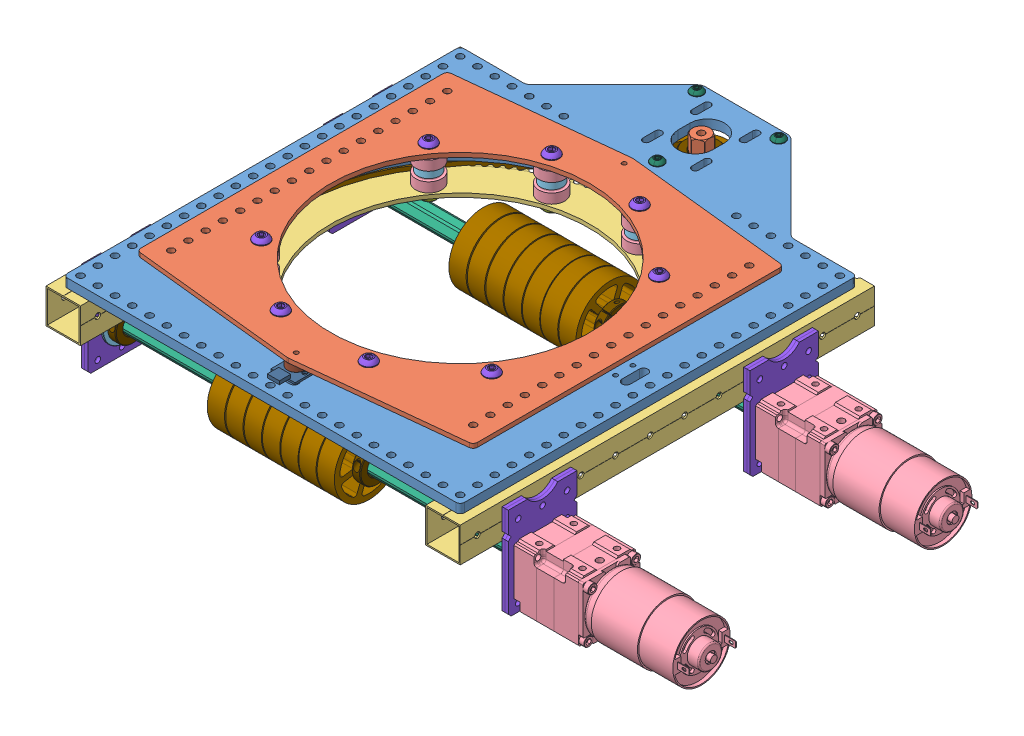
SolidWorks assembly Turret, configuration Default. Lengths in mm.
Overall size (762 1050.2 1114.79).
152 component instances, 28 part files, 7 mates.
Components (placement in the parent):
- Skeleton-1: Skeleton [Default] at origin
- WCP-0280 Rev1 - GreyT Turret-1: WCP-0280 Rev1 - GreyT Turret [Default] at (0 538.7787 -157.715) size (454.1 179.88 363.61)
  - WCP-0280-001 Rev1-1: WCP-0280-001 Rev1 [Default] at origin size (292.1 6.6 356.64)
  - spinner_tray_+_sprocket^WCP-0280 Rev1 - GreyT Turret-1: spinner_tray_+_sprocket^WCP-0280 Rev1 - GreyT Turret [Default] at origin size (248.55 39.23 334.09)
    - WCP-0280-002 Rev1-1: WCP-0280-002 Rev1 [Default] at (0 12.9476 0) size (247.65 3.17 254)
    - WCP-0280-004 Rev1-1: WCP-0280-004 Rev1 [Default] at (0 -14.1605 0) size (246.3 3.25 246.3)
    - bearing_assembly^spinner_tray_+_sprocket-1: bearing_assembly^spinner_tray_+_sprocket [Default] at (-31.5529 25.185 -41.3287) size (26.53 39.23 26.53)
      - WCP-0212_0_250_radial_bearing-1: WCP-0212_0_250_radial_bearing [Default] at (-53.2118 -18.2653 102.9139) x (-0.999427 0 0.033839) z (0 -1 0) size (19.05 19.05 7.14)
      - WCP-0212_0_250_radial_bearing-2: WCP-0212_0_250_radial_bearing [Default] at (-53.2118 -32.1147 102.9139) x (-0.572891 0 0.819632) z (0 1 0) size (19.05 19.05 7.14)
      - WCP-0041_0_250_radial_bearing-1: WCP-0041_0_250_radial_bearing [Default] at (-53.2118 -25.19 102.9139) x (-0.872331 0 0.488916) z (0 -1 0) size (15.88 15.88 4.98)
      - NFS-0011_0_250ID_fiber_washer_95601A310-1: NFS-0011_0_250ID_fiber_washer_95601A310 [Default] at (-53.2118 -35.6866 102.9139) x (0 -1 0) z (-0.326131 0 -0.945325) size (0.86 9.53 9.53)
      - NFS-0011_0_250ID_fiber_washer_95601A310-2: NFS-0011_0_250ID_fiber_washer_95601A310 [Default] at (-53.2118 -22.7008 102.9139) x (0 1 0) z (-0.943269 0 0.332029) size (0.86 9.53 9.53)
      - NFS-0011_0_250ID_fiber_washer_95601A310-3: NFS-0011_0_250ID_fiber_washer_95601A310 [Default] at (-53.2118 -28.5428 102.9139) x (0 1 0) z (-0.160822 0 -0.986983) size (0.86 9.53 9.53)
      - NFS-0011_0_250ID_fiber_washer_95601A310-4: NFS-0011_0_250ID_fiber_washer_95601A310 [Default] at (-53.2118 -14.6935 102.9139) x (0 1 0) z (-0.168532 0 -0.985696) size (0.86 9.53 9.53)
      - NFS-0024_250-20_thin_locknut_90566A029-1: NFS-0024_250-20_thin_locknut_90566A029 [Default] at (-53.2118 -39.3502 102.9139) x (0.28034 0 -0.959901) z (-0.959901 0 -0.28034) size (11.11 5.35 12.83)
      - NFS-0057_SHCS_250-20_1_375L_91255A526-1: NFS-0057_SHCS_250-20_1_375L_91255A526 [Default] at (-53.2118 -7.2971 102.9139) x (0.67695 0 0.736029) z (0 1 0) size (11.17 11.22 39.23)
    - WCP-0280-005 Rev1-1: WCP-0280-005 Rev1 [Default] at (0 -12.7603 -88.6925) size (248.55 9 320.83)
    - hall_effect_board_WCP-0971-1: hall_effect_board_WCP-0971 [Default] at (-8.89 3.302 116.459) x (-1 0 0) z (0 1 0) size (17.78 21.08 5.08)
    - hall_effect_magnet_WCP-0030-1: hall_effect_magnet_WCP-0030 [Default] at (0 8.8602 120.65) x (0.543179 0 0.839617) z (-0.839617 0 0.543179) size (12.7 5 12.7)
    - bearing_assembly^spinner_tray_+_sprocket-2: bearing_assembly^spinner_tray_+_sprocket [Default] at (-51.901 25.185 -172.6831) x (0.982082 0 -0.188455) z (0.188455 0 0.982082) size (26.53 39.23 26.53)
      - WCP-0212_0_250_radial_bearing-1: WCP-0212_0_250_radial_bearing [Default] at (-53.2118 -18.2653 102.9139) x (-0.999427 0 0.033839) z (0 -1 0) size (19.05 19.05 7.14)
      - WCP-0212_0_250_radial_bearing-2: WCP-0212_0_250_radial_bearing [Default] at (-53.2118 -32.1147 102.9139) x (-0.572891 0 0.819632) z (0 1 0) size (19.05 19.05 7.14)
      - WCP-0041_0_250_radial_bearing-1: WCP-0041_0_250_radial_bearing [Default] at (-53.2118 -25.19 102.9139) x (-0.872331 0 0.488916) z (0 -1 0) size (15.88 15.88 4.98)
      - NFS-0011_0_250ID_fiber_washer_95601A310-1: NFS-0011_0_250ID_fiber_washer_95601A310 [Default] at (-53.2118 -35.6866 102.9139) x (0 -1 0) z (-0.326131 0 -0.945325) size (0.86 9.53 9.53)
      - NFS-0011_0_250ID_fiber_washer_95601A310-2: NFS-0011_0_250ID_fiber_washer_95601A310 [Default] at (-53.2118 -22.7008 102.9139) x (0 1 0) z (-0.943269 0 0.332029) size (0.86 9.53 9.53)
      - NFS-0011_0_250ID_fiber_washer_95601A310-3: NFS-0011_0_250ID_fiber_washer_95601A310 [Default] at (-53.2118 -28.5428 102.9139) x (0 1 0) z (-0.160822 0 -0.986983) size (0.86 9.53 9.53)
      - NFS-0011_0_250ID_fiber_washer_95601A310-4: NFS-0011_0_250ID_fiber_washer_95601A310 [Default] at (-53.2118 -14.6935 102.9139) x (0 1 0) z (-0.168532 0 -0.985696) size (0.86 9.53 9.53)
      - NFS-0024_250-20_thin_locknut_90566A029-1: NFS-0024_250-20_thin_locknut_90566A029 [Default] at (-53.2118 -39.3502 102.9139) x (0.28034 0 -0.959901) z (-0.959901 0 -0.28034) size (11.11 5.35 12.83)
      - NFS-0057_SHCS_250-20_1_375L_91255A526-1: NFS-0057_SHCS_250-20_1_375L_91255A526 [Default] at (-53.2118 -7.2971 102.9139) x (0.67695 0 0.736029) z (0 1 0) size (11.17 11.22 39.23)
    - bearing_assembly^spinner_tray_+_sprocket-3: bearing_assembly^spinner_tray_+_sprocket [Default] at (-24.2359 25.185 -215.2172) x (0.918365 0 -0.395734) z (0.395734 0 0.918365) size (26.53 39.23 26.53)
      - WCP-0212_0_250_radial_bearing-1: WCP-0212_0_250_radial_bearing [Default] at (-53.2118 -18.2653 102.9139) x (-0.999427 0 0.033839) z (0 -1 0) size (19.05 19.05 7.14)
      - WCP-0212_0_250_radial_bearing-2: WCP-0212_0_250_radial_bearing [Default] at (-53.2118 -32.1147 102.9139) x (-0.572891 0 0.819632) z (0 1 0) size (19.05 19.05 7.14)
      - WCP-0041_0_250_radial_bearing-1: WCP-0041_0_250_radial_bearing [Default] at (-53.2118 -25.19 102.9139) x (-0.872331 0 0.488916) z (0 -1 0) size (15.88 15.88 4.98)
      - NFS-0011_0_250ID_fiber_washer_95601A310-1: NFS-0011_0_250ID_fiber_washer_95601A310 [Default] at (-53.2118 -35.6866 102.9139) x (0 -1 0) z (-0.326131 0 -0.945325) size (0.86 9.53 9.53)
      - NFS-0011_0_250ID_fiber_washer_95601A310-2: NFS-0011_0_250ID_fiber_washer_95601A310 [Default] at (-53.2118 -22.7008 102.9139) x (0 1 0) z (-0.943269 0 0.332029) size (0.86 9.53 9.53)
      - NFS-0011_0_250ID_fiber_washer_95601A310-3: NFS-0011_0_250ID_fiber_washer_95601A310 [Default] at (-53.2118 -28.5428 102.9139) x (0 1 0) z (-0.160822 0 -0.986983) size (0.86 9.53 9.53)
      - NFS-0011_0_250ID_fiber_washer_95601A310-4: NFS-0011_0_250ID_fiber_washer_95601A310 [Default] at (-53.2118 -14.6935 102.9139) x (0 1 0) z (-0.168532 0 -0.985696) size (0.86 9.53 9.53)
      - NFS-0024_250-20_thin_locknut_90566A029-1: NFS-0024_250-20_thin_locknut_90566A029 [Default] at (-53.2118 -39.3502 102.9139) x (0.28034 0 -0.959901) z (-0.959901 0 -0.28034) size (11.11 5.35 12.83)
      - NFS-0057_SHCS_250-20_1_375L_91255A526-1: NFS-0057_SHCS_250-20_1_375L_91255A526 [Default] at (-53.2118 -7.2971 102.9139) x (0.67695 0 0.736029) z (0 1 0) size (11.17 11.22 39.23)
    - bearing_assembly^spinner_tray_+_sprocket-4: bearing_assembly^spinner_tray_+_sprocket [Default] at (13.1984 25.185 -213.9052) x (0.8 0 -0.6) z (0.6 0 0.8) size (26.53 39.23 26.53)
      - WCP-0212_0_250_radial_bearing-1: WCP-0212_0_250_radial_bearing [Default] at (-53.2118 -18.2653 102.9139) x (-0.999427 0 0.033839) z (0 -1 0) size (19.05 19.05 7.14)
      - WCP-0212_0_250_radial_bearing-2: WCP-0212_0_250_radial_bearing [Default] at (-53.2118 -32.1147 102.9139) x (-0.572891 0 0.819632) z (0 1 0) size (19.05 19.05 7.14)
      - WCP-0041_0_250_radial_bearing-1: WCP-0041_0_250_radial_bearing [Default] at (-53.2118 -25.19 102.9139) x (-0.872331 0 0.488916) z (0 -1 0) size (15.88 15.88 4.98)
      - NFS-0011_0_250ID_fiber_washer_95601A310-1: NFS-0011_0_250ID_fiber_washer_95601A310 [Default] at (-53.2118 -35.6866 102.9139) x (0 -1 0) z (-0.326131 0 -0.945325) size (0.86 9.53 9.53)
      - NFS-0011_0_250ID_fiber_washer_95601A310-2: NFS-0011_0_250ID_fiber_washer_95601A310 [Default] at (-53.2118 -22.7008 102.9139) x (0 1 0) z (-0.943269 0 0.332029) size (0.86 9.53 9.53)
      - NFS-0011_0_250ID_fiber_washer_95601A310-3: NFS-0011_0_250ID_fiber_washer_95601A310 [Default] at (-53.2118 -28.5428 102.9139) x (0 1 0) z (-0.160822 0 -0.986983) size (0.86 9.53 9.53)
      - NFS-0011_0_250ID_fiber_washer_95601A310-4: NFS-0011_0_250ID_fiber_washer_95601A310 [Default] at (-53.2118 -14.6935 102.9139) x (0 1 0) z (-0.168532 0 -0.985696) size (0.86 9.53 9.53)
      - NFS-0024_250-20_thin_locknut_90566A029-1: NFS-0024_250-20_thin_locknut_90566A029 [Default] at (-53.2118 -39.3502 102.9139) x (0.28034 0 -0.959901) z (-0.959901 0 -0.28034) size (11.11 5.35 12.83)
      - NFS-0057_SHCS_250-20_1_375L_91255A526-1: NFS-0057_SHCS_250-20_1_375L_91255A526 [Default] at (-53.2118 -7.2971 102.9139) x (0.67695 0 0.736029) z (0 1 0) size (11.17 11.22 39.23)
    - bearing_assembly^spinner_tray_+_sprocket-5: bearing_assembly^spinner_tray_+_sprocket [Default] at (38.8565 25.185 -167.9581) x (0.63358 0 -0.773678) z (0.773678 0 0.63358) size (26.53 39.23 26.53)
      - WCP-0212_0_250_radial_bearing-1: WCP-0212_0_250_radial_bearing [Default] at (-53.2118 -18.2653 102.9139) x (-0.999427 0 0.033839) z (0 -1 0) size (19.05 19.05 7.14)
      - WCP-0212_0_250_radial_bearing-2: WCP-0212_0_250_radial_bearing [Default] at (-53.2118 -32.1147 102.9139) x (-0.572891 0 0.819632) z (0 1 0) size (19.05 19.05 7.14)
      - WCP-0041_0_250_radial_bearing-1: WCP-0041_0_250_radial_bearing [Default] at (-53.2118 -25.19 102.9139) x (-0.872331 0 0.488916) z (0 -1 0) size (15.88 15.88 4.98)
      - NFS-0011_0_250ID_fiber_washer_95601A310-1: NFS-0011_0_250ID_fiber_washer_95601A310 [Default] at (-53.2118 -35.6866 102.9139) x (0 -1 0) z (-0.326131 0 -0.945325) size (0.86 9.53 9.53)
      - NFS-0011_0_250ID_fiber_washer_95601A310-2: NFS-0011_0_250ID_fiber_washer_95601A310 [Default] at (-53.2118 -22.7008 102.9139) x (0 1 0) z (-0.943269 0 0.332029) size (0.86 9.53 9.53)
      - NFS-0011_0_250ID_fiber_washer_95601A310-3: NFS-0011_0_250ID_fiber_washer_95601A310 [Default] at (-53.2118 -28.5428 102.9139) x (0 1 0) z (-0.160822 0 -0.986983) size (0.86 9.53 9.53)
      - NFS-0011_0_250ID_fiber_washer_95601A310-4: NFS-0011_0_250ID_fiber_washer_95601A310 [Default] at (-53.2118 -14.6935 102.9139) x (0 1 0) z (-0.168532 0 -0.985696) size (0.86 9.53 9.53)
      - NFS-0024_250-20_thin_locknut_90566A029-1: NFS-0024_250-20_thin_locknut_90566A029 [Default] at (-53.2118 -39.3502 102.9139) x (0.28034 0 -0.959901) z (-0.959901 0 -0.28034) size (11.11 5.35 12.83)
      - NFS-0057_SHCS_250-20_1_375L_91255A526-1: NFS-0057_SHCS_250-20_1_375L_91255A526 [Default] at (-53.2118 -7.2971 102.9139) x (0.67695 0 0.736029) z (0 1 0) size (11.17 11.22 39.23)
    - bearing_assembly^spinner_tray_+_sprocket-6: bearing_assembly^spinner_tray_+_sprocket [Default] at (16.1385 25.185 -31.7594) x (0.443629 0 -0.896211) z (0.896211 0 0.443629) size (26.53 39.23 26.53)
      - WCP-0212_0_250_radial_bearing-1: WCP-0212_0_250_radial_bearing [Default] at (-53.2118 -18.2653 102.9139) x (-0.999427 0 0.033839) z (0 -1 0) size (19.05 19.05 7.14)
      - WCP-0212_0_250_radial_bearing-2: WCP-0212_0_250_radial_bearing [Default] at (-53.2118 -32.1147 102.9139) x (-0.572891 0 0.819632) z (0 1 0) size (19.05 19.05 7.14)
      - WCP-0041_0_250_radial_bearing-1: WCP-0041_0_250_radial_bearing [Default] at (-53.2118 -25.19 102.9139) x (-0.872331 0 0.488916) z (0 -1 0) size (15.88 15.88 4.98)
      - NFS-0011_0_250ID_fiber_washer_95601A310-1: NFS-0011_0_250ID_fiber_washer_95601A310 [Default] at (-53.2118 -35.6866 102.9139) x (0 -1 0) z (-0.326131 0 -0.945325) size (0.86 9.53 9.53)
      - NFS-0011_0_250ID_fiber_washer_95601A310-2: NFS-0011_0_250ID_fiber_washer_95601A310 [Default] at (-53.2118 -22.7008 102.9139) x (0 1 0) z (-0.943269 0 0.332029) size (0.86 9.53 9.53)
      - NFS-0011_0_250ID_fiber_washer_95601A310-3: NFS-0011_0_250ID_fiber_washer_95601A310 [Default] at (-53.2118 -28.5428 102.9139) x (0 1 0) z (-0.160822 0 -0.986983) size (0.86 9.53 9.53)
      - NFS-0011_0_250ID_fiber_washer_95601A310-4: NFS-0011_0_250ID_fiber_washer_95601A310 [Default] at (-53.2118 -14.6935 102.9139) x (0 1 0) z (-0.168532 0 -0.985696) size (0.86 9.53 9.53)
      - NFS-0024_250-20_thin_locknut_90566A029-1: NFS-0024_250-20_thin_locknut_90566A029 [Default] at (-53.2118 -39.3502 102.9139) x (0.28034 0 -0.959901) z (-0.959901 0 -0.28034) size (11.11 5.35 12.83)
      - NFS-0057_SHCS_250-20_1_375L_91255A526-1: NFS-0057_SHCS_250-20_1_375L_91255A526 [Default] at (-53.2118 -7.2971 102.9139) x (0.67695 0 0.736029) z (0 1 0) size (11.17 11.22 39.23)
    - bearing_assembly^spinner_tray_+_sprocket-7: bearing_assembly^spinner_tray_+_sprocket [Default] at (-52.9007 25.185 21.2222) x (0.263225 0 -0.964735) z (0.964735 0 0.263225) size (26.53 39.23 26.53)
      - WCP-0212_0_250_radial_bearing-1: WCP-0212_0_250_radial_bearing [Default] at (-53.2118 -18.2653 102.9139) x (-0.999427 0 0.033839) z (0 -1 0) size (19.05 19.05 7.14)
      - WCP-0212_0_250_radial_bearing-2: WCP-0212_0_250_radial_bearing [Default] at (-53.2118 -32.1147 102.9139) x (-0.572891 0 0.819632) z (0 1 0) size (19.05 19.05 7.14)
      - WCP-0041_0_250_radial_bearing-1: WCP-0041_0_250_radial_bearing [Default] at (-53.2118 -25.19 102.9139) x (-0.872331 0 0.488916) z (0 -1 0) size (15.88 15.88 4.98)
      - NFS-0011_0_250ID_fiber_washer_95601A310-1: NFS-0011_0_250ID_fiber_washer_95601A310 [Default] at (-53.2118 -35.6866 102.9139) x (0 -1 0) z (-0.326131 0 -0.945325) size (0.86 9.53 9.53)
      - NFS-0011_0_250ID_fiber_washer_95601A310-2: NFS-0011_0_250ID_fiber_washer_95601A310 [Default] at (-53.2118 -22.7008 102.9139) x (0 1 0) z (-0.943269 0 0.332029) size (0.86 9.53 9.53)
      - NFS-0011_0_250ID_fiber_washer_95601A310-3: NFS-0011_0_250ID_fiber_washer_95601A310 [Default] at (-53.2118 -28.5428 102.9139) x (0 1 0) z (-0.160822 0 -0.986983) size (0.86 9.53 9.53)
      - NFS-0011_0_250ID_fiber_washer_95601A310-4: NFS-0011_0_250ID_fiber_washer_95601A310 [Default] at (-53.2118 -14.6935 102.9139) x (0 1 0) z (-0.168532 0 -0.985696) size (0.86 9.53 9.53)
      - NFS-0024_250-20_thin_locknut_90566A029-1: NFS-0024_250-20_thin_locknut_90566A029 [Default] at (-53.2118 -39.3502 102.9139) x (0.28034 0 -0.959901) z (-0.959901 0 -0.28034) size (11.11 5.35 12.83)
      - NFS-0057_SHCS_250-20_1_375L_91255A526-1: NFS-0057_SHCS_250-20_1_375L_91255A526 [Default] at (-53.2118 -7.2971 102.9139) x (0.67695 0 0.736029) z (0 1 0) size (11.17 11.22 39.23)
    - bearing_assembly^spinner_tray_+_sprocket-8: bearing_assembly^spinner_tray_+_sprocket [Default] at (-128.1504 25.185 34.4528) x (0.120178 0 -0.992752) z (0.992752 0 0.120178) size (26.53 39.23 26.53)
      - WCP-0212_0_250_radial_bearing-1: WCP-0212_0_250_radial_bearing [Default] at (-53.2118 -18.2653 102.9139) x (-0.999427 0 0.033839) z (0 -1 0) size (19.05 19.05 7.14)
      - WCP-0212_0_250_radial_bearing-2: WCP-0212_0_250_radial_bearing [Default] at (-53.2118 -32.1147 102.9139) x (-0.572891 0 0.819632) z (0 1 0) size (19.05 19.05 7.14)
      - WCP-0041_0_250_radial_bearing-1: WCP-0041_0_250_radial_bearing [Default] at (-53.2118 -25.19 102.9139) x (-0.872331 0 0.488916) z (0 -1 0) size (15.88 15.88 4.98)
      - NFS-0011_0_250ID_fiber_washer_95601A310-1: NFS-0011_0_250ID_fiber_washer_95601A310 [Default] at (-53.2118 -35.6866 102.9139) x (0 -1 0) z (-0.326131 0 -0.945325) size (0.86 9.53 9.53)
      - NFS-0011_0_250ID_fiber_washer_95601A310-2: NFS-0011_0_250ID_fiber_washer_95601A310 [Default] at (-53.2118 -22.7008 102.9139) x (0 1 0) z (-0.943269 0 0.332029) size (0.86 9.53 9.53)
      - NFS-0011_0_250ID_fiber_washer_95601A310-3: NFS-0011_0_250ID_fiber_washer_95601A310 [Default] at (-53.2118 -28.5428 102.9139) x (0 1 0) z (-0.160822 0 -0.986983) size (0.86 9.53 9.53)
      - NFS-0011_0_250ID_fiber_washer_95601A310-4: NFS-0011_0_250ID_fiber_washer_95601A310 [Default] at (-53.2118 -14.6935 102.9139) x (0 1 0) z (-0.168532 0 -0.985696) size (0.86 9.53 9.53)
      - NFS-0024_250-20_thin_locknut_90566A029-1: NFS-0024_250-20_thin_locknut_90566A029 [Default] at (-53.2118 -39.3502 102.9139) x (0.28034 0 -0.959901) z (-0.959901 0 -0.28034) size (11.11 5.35 12.83)
      - NFS-0057_SHCS_250-20_1_375L_91255A526-1: NFS-0057_SHCS_250-20_1_375L_91255A526 [Default] at (-53.2118 -7.2971 102.9139) x (0.67695 0 0.736029) z (0 1 0) size (11.17 11.22 39.23)
  - turret_swivel_motor_assembly^WCP-0280 Rev1 - GreyT Turret-1: turret_swivel_motor_assembly^WCP-0280 Rev1 - GreyT Turret [Default] at origin size (73.41 167.54 80.86)
    - WCP-0280-003 Rev1-1: WCP-0280-003 Rev1 [Default] at (0 -33.4645 -177.3845) size (73.03 3.17 73.44)
    - wcd_cam_217-3431-1: wcd_cam_217-3431 [Default] at (-2.1071 -41.402 -145.7696) x (0.727312 0 -0.686307) z (0 -1 0) size (22.69 21.26 12.7)
    - WCP-0226 Rev1-1: WCP-0226 Rev1 [Default] at (30.1625 -17.5895 -204.235) x (0 1 0) z (-0.493388 0 0.869809) size (28.57 9.5 9.5)
    - WCP-0226 Rev1-2: WCP-0226 Rev1 [Default] at (0 -17.5895 -145.0815) x (0 1 0) z (-0.104761 0 0.994497) size (28.57 9.5 9.5)
    - WCP-0226 Rev1-3: WCP-0226 Rev1 [Default] at (-30.1625 -17.5895 -204.235) x (0 1 0) z (-0.104761 0 0.994497) size (28.57 9.5 9.5)
    - WCP-0258 Rev1-1: WCP-0258 Rev1 [Default] at (0 5.8674 -145.0815) x (0.945142 0 -0.32666) z (0 1 0) size (9.2 9.23 49.52)
    - WCP-0258 Rev1-2: WCP-0258 Rev1 [Default] at (-30.1625 5.8674 -204.235) x (0.945142 0 -0.32666) z (0 1 0) size (9.2 9.23 49.52)
    - WCP-0258 Rev1-3: WCP-0258 Rev1 [Default] at (30.1625 5.8674 -204.235) x (0.945142 0 -0.32666) z (0 1 0) size (9.2 9.23 49.52)
    - NFS-0010_#10-32_thin_locknut_Default_As Machined_-1: NFS-0010_#10-32_thin_locknut_Default_As Machined_ [Default] at (-30.1625 -35.052 -204.235) x (0.910739 0 -0.412983) z (-0.412983 0 -0.910739) size (9.53 4.37 11)
    - NFS-0010_#10-32_thin_locknut_Default_As Machined_-2: NFS-0010_#10-32_thin_locknut_Default_As Machined_ [Default] at (30.1625 -35.052 -204.235) x (-0.933743 0 -0.357945) z (-0.357945 0 0.933743) size (9.53 4.37 11)
    - WCP-0253 Rev1-1: WCP-0253 Rev1 [Default] at (17.9605 -29.3116 -159.4245) x (0.553393 0 -0.83292) z (0 1 0) size (9.24 9.28 15.9)
    - WCP-0253 Rev1-2: WCP-0253 Rev1 [Default] at (-17.9605 -29.3116 -195.3456) x (-0.735473 0 -0.677555) z (0 1 0) size (9.24 9.28 15.9)
    - 217-2737_500_hex_collar-1: 217-2737_500_hex_collar [Default] at (0 -23.7141 -177.3851) x (0.975283 0 0.220959) z (0 1 0) size (25.39 25.4 7.82)
    - 217-2737_500_hex_collar-2: 217-2737_500_hex_collar [Default] at (0 -8.1883 -177.3851) x (0.855545 0 0.517728) z (0 -1 0) size (25.39 25.4 7.82)
    - 217-2642_16T_500_hex-1: 217-2642_16T_500_hex [Default] at (0 -14.1573 -177.3851) x (0.551766 0 -0.833999) z (0 1 0) size (35.21 35.21 9.18)
    - v2_versa_planetary_1_stage-1: v2_versa_planetary_1_stage [Default] at (22.225 -51.677 -177.3851) x (0 1 0) z (0 0 1) size (166.6 44.45 44.3)
  - 1x1_tube_stock_WCP-0280-006 Rev1-1: 1x1_tube_stock_WCP-0280-006 Rev1 [Default] at (139.7 -16.002 -596.9) size (25.4 25.4 304.8)
  - 1x1_tube_stock_WCP-0280-006 Rev1-2: 1x1_tube_stock_WCP-0280-006 Rev1 [Default] at (-139.7 -16.002 -596.9) size (25.4 25.4 304.8)
  - pre-roller_assembly-1: pre-roller_assembly [Default] at origin size (454.1 80.43 71.81)
    - v2_versa_planetary_1_stage_no_output-1: v2_versa_planetary_1_stage_no_output [Default] at (173.597 -73.6827 96.3395) x (-1 0 0) z (0 0 -1) size (126.03 44.45 44.3)
    - 217-4006_0_500_flanged_thunderhex_bearing-1: 217-4006_0_500_flanged_thunderhex_bearing [Default] at (-154.7812 -51.4577 96.3395) x (0 -0.481649 -0.876364) z (1 0 0) size (31.12 31.12 7.94)
    - WCP-0280-007 Rev1-1: WCP-0280-007 Rev1 [Default] at (-12.3532 -51.4577 96.3395) x (1 0 0) z (0 -0.918939 0.3944) size (317.5 12.7 13.75)
    - WCP-0253 Rev1-1: WCP-0253 Rev1 [Default] at (149.8346 -69.4182 78.379) x (0 -0.851264 -0.524738) z (-1 0 0) size (9.24 9.28 15.9)
    - WCP-0253 Rev1-2: WCP-0253 Rev1 [Default] at (149.8346 -33.4972 114.3) x (0 0.557595 -0.830113) z (-1 0 0) size (9.24 9.28 15.9)
    - 217-2737_500_hex_collar-1: 217-2737_500_hex_collar [Default] at (-161.925 -51.4577 96.3395) x (0 0.97196 0.235146) z (1 0 0) size (25.39 25.4 7.82)
    - 217-2737_500_hex_collar-2: 217-2737_500_hex_collar [Default] at (-147.6375 -51.4577 96.3395) x (0 0.799523 0.600635) z (-1 0 0) size (25.39 25.4 7.82)
    - Universal_Female_Output_Shaft_1_2_Hex-1: Universal_Female_Output_Shaft_1_2_Hex [Default] at (166.1492 -51.4577 96.3395) x (0 0.997742 0.067166) z (-1 0 0) size (21.37 20 42.62)
    - 217-4183_VersaFrame_Face_Bearing_Mount-1: 217-4183_VersaFrame_Face_Bearing_Mount [Default] at (154.686 -24.7496 96.3395) x (0 -1 0) z (1 0 0) size (68.49 50.55 2.29)
    - 217-4183_VersaFrame_Face_Bearing_Mount-2: 217-4183_VersaFrame_Face_Bearing_Mount [Default] at (152.4 -24.7496 96.3395) x (0 -1 0) z (1 0 0) size (68.49 50.55 2.29)
    - 217-4183_VersaFrame_Face_Bearing_Mount-3: 217-4183_VersaFrame_Face_Bearing_Mount [Default] at (-154.686 -24.7496 96.3395) x (0 -1 0) z (1 0 0) size (68.49 50.55 2.29)
    - 217-4183_VersaFrame_Face_Bearing_Mount-4: 217-4183_VersaFrame_Face_Bearing_Mount [Default] at (-156.972 -24.7496 96.3395) x (0 -1 0) z (1 0 0) size (68.49 50.55 2.29)
    - 2_OD_Straight_Flex_Wheel_217-6446-1: 2_OD_Straight_Flex_Wheel_217-6446 [Default] at (9.3117 -51.4577 96.3395) x (0 0.610406 -0.792088) z (0 0.792088 0.610406) size (50.8 12.7 50.8)
    - 2_OD_Straight_Flex_Wheel_217-6446-2: 2_OD_Straight_Flex_Wheel_217-6446 [Default] at (-58.0571 -51.4577 96.3395) x (0 0.249738 -0.968314) z (0 0.968314 0.249738) size (50.8 12.7 50.8)
    - 2_OD_Straight_Flex_Wheel_217-6446-3: 2_OD_Straight_Flex_Wheel_217-6446 [Default] at (-3.9428 -51.4577 96.3395) x (0 -0.070457 -0.997515) z (0 0.997515 -0.070457) size (50.8 12.7 50.8)
    - 217-2737_500_hex_collar-3: 217-2737_500_hex_collar [Default] at (32.3405 -51.4577 96.3395) x (0 0.832718 0.553698) z (-1 0 0) size (25.39 25.4 7.82)
    - 217-2737_500_hex_collar-4: 217-2737_500_hex_collar [Default] at (-68.0772 -51.4577 96.3395) x (0 0.724871 0.688884) z (-1 0 0) size (25.39 25.4 7.82)
    - 2_OD_Straight_Flex_Wheel_217-6446-4: 2_OD_Straight_Flex_Wheel_217-6446 [Default] at (-30.9117 -51.4577 96.3395) x (0 0.410417 -0.911898) z (0 0.911898 0.410417) size (50.8 12.7 50.8)
    - 2_OD_Straight_Flex_Wheel_217-6446-5: 2_OD_Straight_Flex_Wheel_217-6446 [Default] at (-17.4177 -51.4577 96.3395) x (0 0.496878 -0.86782) z (0 0.86782 0.496878) size (50.8 12.7 50.8)
    - 2_OD_Straight_Flex_Wheel_217-6446-6: 2_OD_Straight_Flex_Wheel_217-6446 [Default] at (-44.4634 -51.4577 96.3395) x (0 0.687316 -0.726359) z (0 0.726359 0.687316) size (50.8 12.7 50.8)
    - 2_OD_Straight_Flex_Wheel_217-6446-7: 2_OD_Straight_Flex_Wheel_217-6446 [Default] at (22.7808 -51.4577 96.3395) x (0 0.629554 -0.776957) z (0 0.776957 0.629554) size (50.8 12.7 50.8)
  - pre-roller_assembly-2: pre-roller_assembly [Default] at (0 0 -177.8) size (454.1 80.43 71.81)
    - v2_versa_planetary_1_stage_no_output-1: v2_versa_planetary_1_stage_no_output [Default] at (173.597 -73.6827 96.3395) x (-1 0 0) z (0 0 -1) size (126.03 44.45 44.3)
    - 217-4006_0_500_flanged_thunderhex_bearing-1: 217-4006_0_500_flanged_thunderhex_bearing [Default] at (-154.7812 -51.4577 96.3395) x (0 -0.481649 -0.876364) z (1 0 0) size (31.12 31.12 7.94)
    - WCP-0280-007 Rev1-1: WCP-0280-007 Rev1 [Default] at (-12.3532 -51.4577 96.3395) x (1 0 0) z (0 -0.918939 0.3944) size (317.5 12.7 13.75)
    - WCP-0253 Rev1-1: WCP-0253 Rev1 [Default] at (149.8346 -69.4182 78.379) x (0 -0.851264 -0.524738) z (-1 0 0) size (9.24 9.28 15.9)
    - WCP-0253 Rev1-2: WCP-0253 Rev1 [Default] at (149.8346 -33.4972 114.3) x (0 0.557595 -0.830113) z (-1 0 0) size (9.24 9.28 15.9)
    - 217-2737_500_hex_collar-1: 217-2737_500_hex_collar [Default] at (-161.925 -51.4577 96.3395) x (0 0.97196 0.235146) z (1 0 0) size (25.39 25.4 7.82)
    - 217-2737_500_hex_collar-2: 217-2737_500_hex_collar [Default] at (-147.6375 -51.4577 96.3395) x (0 0.799523 0.600635) z (-1 0 0) size (25.39 25.4 7.82)
    - Universal_Female_Output_Shaft_1_2_Hex-1: Universal_Female_Output_Shaft_1_2_Hex [Default] at (166.1492 -51.4577 96.3395) x (0 0.997742 0.067166) z (-1 0 0) size (21.37 20 42.62)
    - 217-4183_VersaFrame_Face_Bearing_Mount-1: 217-4183_VersaFrame_Face_Bearing_Mount [Default] at (154.686 -24.7496 96.3395) x (0 -1 0) z (1 0 0) size (68.49 50.55 2.29)
    - 217-4183_VersaFrame_Face_Bearing_Mount-2: 217-4183_VersaFrame_Face_Bearing_Mount [Default] at (152.4 -24.7496 96.3395) x (0 -1 0) z (1 0 0) size (68.49 50.55 2.29)
    - 217-4183_VersaFrame_Face_Bearing_Mount-3: 217-4183_VersaFrame_Face_Bearing_Mount [Default] at (-154.686 -24.7496 96.3395) x (0 -1 0) z (1 0 0) size (68.49 50.55 2.29)
    - 217-4183_VersaFrame_Face_Bearing_Mount-4: 217-4183_VersaFrame_Face_Bearing_Mount [Default] at (-156.972 -24.7496 96.3395) x (0 -1 0) z (1 0 0) size (68.49 50.55 2.29)
    - 2_OD_Straight_Flex_Wheel_217-6446-1: 2_OD_Straight_Flex_Wheel_217-6446 [Default] at (9.3117 -51.4577 96.3395) x (0 0.610406 -0.792088) z (0 0.792088 0.610406) size (50.8 12.7 50.8)
    - 2_OD_Straight_Flex_Wheel_217-6446-2: 2_OD_Straight_Flex_Wheel_217-6446 [Default] at (-58.0571 -51.4577 96.3395) x (0 0.249738 -0.968314) z (0 0.968314 0.249738) size (50.8 12.7 50.8)
    - 2_OD_Straight_Flex_Wheel_217-6446-3: 2_OD_Straight_Flex_Wheel_217-6446 [Default] at (-3.9428 -51.4577 96.3395) x (0 -0.070457 -0.997515) z (0 0.997515 -0.070457) size (50.8 12.7 50.8)
    - 217-2737_500_hex_collar-3: 217-2737_500_hex_collar [Default] at (32.3405 -51.4577 96.3395) x (0 0.832718 0.553698) z (-1 0 0) size (25.39 25.4 7.82)
    - 217-2737_500_hex_collar-4: 217-2737_500_hex_collar [Default] at (-68.0772 -51.4577 96.3395) x (0 0.724871 0.688884) z (-1 0 0) size (25.39 25.4 7.82)
    - 2_OD_Straight_Flex_Wheel_217-6446-4: 2_OD_Straight_Flex_Wheel_217-6446 [Default] at (-30.9117 -51.4577 96.3395) x (0 0.410417 -0.911898) z (0 0.911898 0.410417) size (50.8 12.7 50.8)
    - 2_OD_Straight_Flex_Wheel_217-6446-5: 2_OD_Straight_Flex_Wheel_217-6446 [Default] at (-17.4177 -51.4577 96.3395) x (0 0.496878 -0.86782) z (0 0.86782 0.496878) size (50.8 12.7 50.8)
    - 2_OD_Straight_Flex_Wheel_217-6446-6: 2_OD_Straight_Flex_Wheel_217-6446 [Default] at (-44.4634 -51.4577 96.3395) x (0 0.687316 -0.726359) z (0 0.726359 0.687316) size (50.8 12.7 50.8)
    - 2_OD_Straight_Flex_Wheel_217-6446-7: 2_OD_Straight_Flex_Wheel_217-6446 [Default] at (22.7808 -51.4577 96.3395) x (0 0.629554 -0.776957) z (0 0.776957 0.629554) size (50.8 12.7 50.8)
Mates (geometry in assembly coordinates):
- Coincident2: coincident aligned: plane of Skeleton-1 through (0 0 0) normal (0 0 1)
- Coincident3: coincident aligned: plane of Skeleton-1 through (0 0 0) normal (0 1 0)
- Coincident4: coincident aligned: plane of Skeleton-1 through (0 0 0) normal (1 0 0)
- Coincident5: coincident aligned: plane of Skeleton-1 through (0 553.3138 0) normal (0 1 0); plane of WCP-0280 Rev1 - GreyT Turret-1/WCP-0280-002 Rev1-1 through (0 511.1498 -157.715) normal (0 1 0)
- Coincident6: coincident: line of Skeleton-1 through (-152.4 553.3138 -5.315) axis (1 0 0); plane of WCP-0280 Rev1 - GreyT Turret-1/1x1_tube_stock_WCP-0280-006 Rev1-1 through (139.7 522.7767 -5.315) normal (0 0 1)
- Coincident7: coincident: line of Skeleton-1 through (152.4 553.3138 -368.3) axis (0 0 1); plane of WCP-0280 Rev1 - GreyT Turret-1/1x1_tube_stock_WCP-0280-006 Rev1-1 through (152.4 510.0767 -5.315) normal (1 0 0)
- Coincident8: coincident aligned: plane of Skeleton-1 through (0 553.3138 0) normal (0 1 0); plane of WCP-0280 Rev1 - GreyT Turret-1/spinner_tray_+_sprocket^WCP-0280 Rev1 - GreyT Turret-1/WCP-0280-002 Rev1-1 through (0 553.3138 -157.715) normal (0 1 0)
